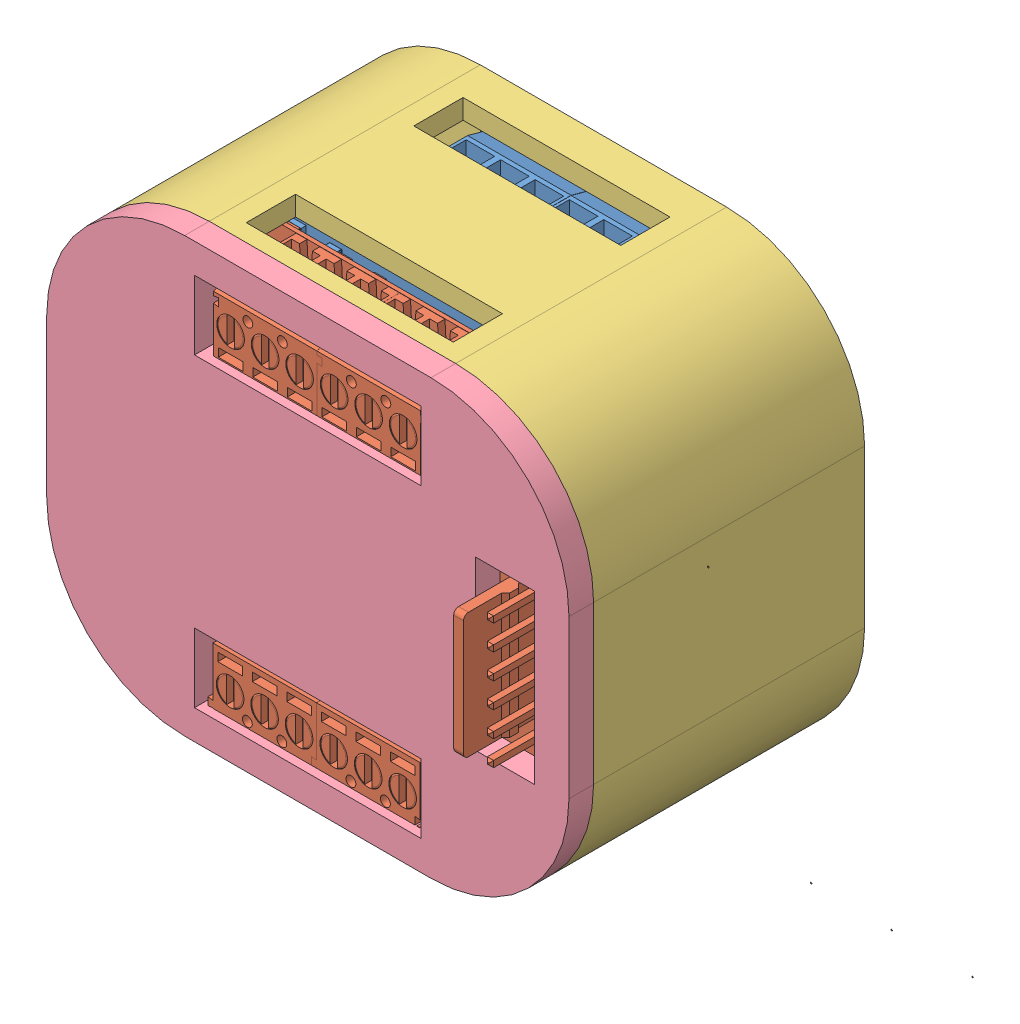
SolidWorks assembly Сборка плат смарт-бокса (утолщ стенки), configuration Default. Lengths in mm.
Overall size (85.93 44 32.41).
4 component instances, 4 part files, 9 mates.
Components (placement in the parent):
- Плата смарт-бокса 1-1: Плата смарт-бокса 1 [Default] at (-165.9192 -27.3465 18.5165) size (50.47 38.8 18.8)
- Плата смарт-бокса 2-1: Плата смарт-бокса 2 [Default] at (-116.116 -27.2195 30.3365) x (1 0 0) z (0 0 1) size (83.29 38.85 21.16)
- Корпус для смарт-бокса, новая версия-2: Корпус для смарт-бокса, новая версия [Default] at (-31.0453 -1.8751 23.405) x (1 0 0) z (0 -1 0) size (53 27.5 44)
- Смарт-бокс, крышка-1: Смарт-бокс, крышка [Default] at (-31.0453 -1.8751 37.155) x (1 0 0) z (0 -1 0) size (53 5 44)
Mates (geometry in assembly coordinates):
- Coincident1: coincident anti-aligned: plane of Плата смарт-бокса 1-1 through (-53.5496 4.7591 26.877) normal (0 0 1); plane of Плата смарт-бокса 2-1 through (-54.7496 6.0291 26.877) normal (0 0 -1)
- Coincident2: coincident aligned: plane of Плата смарт-бокса 1-1 through (-54.7496 6.0291 18.477) normal (0 1 0); plane of Плата смарт-бокса 2-1 through (-53.4796 6.0291 28.147) normal (0 1 0)
- Coincident3: coincident aligned: plane of Плата смарт-бокса 1-1 through (-54.7496 3.4891 18.477) normal (-1 0 0); plane of Плата смарт-бокса 2-1 through (-54.7496 6.0291 29.417) normal (-1 0 0)
- Coincident9: coincident anti-aligned: plane of Корпус для смарт-бокса, новая версия-2 through (-43.5453 6.1249 37.155) normal (0 0 1); plane of Смарт-бокс, крышка-1 through (-43.5453 6.1249 37.155) normal (0 0 -1)
- Coincident10: coincident aligned: plane of Плата смарт-бокса 1-1 through (-20.5577 16.5413 9.655) normal (0 0 -1); plane of Корпус для смарт-бокса, новая версия-2 through (-43.5453 6.1249 9.655) normal (0 0 -1)
- Width2: width aligned: plane of Корпус для смарт-бокса, новая версия-2 through (-20.5453 18.1249 18.405) normal (-1 0 0); plane of Плата смарт-бокса 1-1 through (-41.5453 18.1249 18.405) normal (1 0 0); plane of Корпус для смарт-бокса, новая версия-2 through (-20.8577 11.0413 13.405) normal (-1 0 0); plane of Плата смарт-бокса 1-1 through (-41.2329 11.0634 17.305) normal (1 0 0)
- Distance2: distance = 1.75 mm: point of Плата смарт-бокса 2-1; plane of Корпус для смарт-бокса, новая версия-2 through (-43.5453 -23.8751 37.155) normal (0 -1 0)
- Coincident12: coincident aligned: plane of Корпус для смарт-бокса, новая версия-2 through (-43.5453 -23.8751 37.155) normal (0 -1 0); plane of Смарт-бокс, крышка-1 through (-43.5453 -23.8751 39.655) normal (0 -1 0)
- Coincident13: coincident aligned: plane of Корпус для смарт-бокса, новая версия-2 through (-57.5453 6.1249 37.155) normal (-1 0 0); plane of Смарт-бокс, крышка-1 through (-57.5453 6.1249 39.655) normal (-1 0 0)
